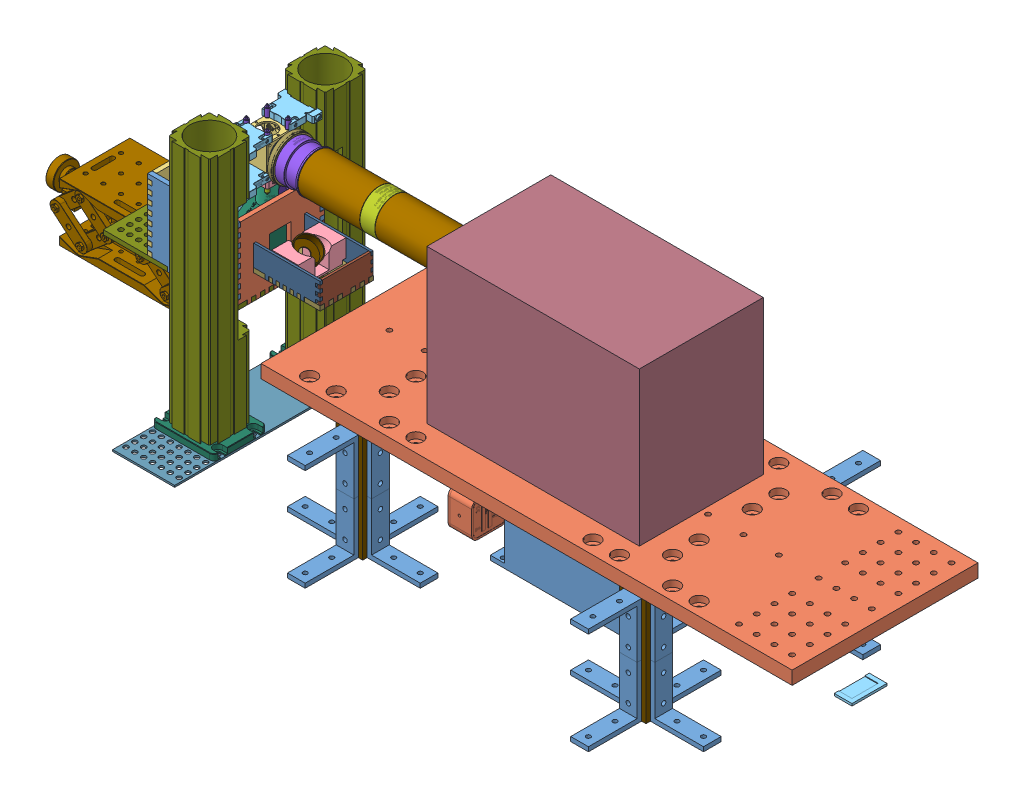
SolidWorks assembly Assembly4, configuration Default. Lengths in mm.
Overall size (1118.21 392.76 419.1).
142 component instances, 57 part files, 22 mates.
Components (placement in the parent):
- Laser Sub-Assembly-1: Laser Sub-Assembly [Default] at (5.2061 -104.2543 0) x (0 0 -1) z (1 0 0) size (111.76 88.9 267.97)
  - Laser-1: Laser [Default] at (0 -56.1594 0) x (0 0 1) z (-1 0 0) size (267.97 88.9 88.9)
  - SH05-Solidworks-1: SH05-Solidworks [Default] at (-45.783 38.7485 -122.8155) x (0 1 0) z (0 0 -1) size (57.1 81.96 34.87)
- Objective Sub-Assembly-1: Objective Sub-Assembly [Default] at (-505.0208 -286.1894 -114.3818) x (0 0 1) z (0 -1 0) size (106.71 57.63 128.02)
  - CM1-DCH-Solidworks-1: CM1-DCH-Solidworks [Web Assembly] at (114.3818 -34.6924 -438.5894) x (0 -1 0) z (0 0 1) size (38.1 45.72 38.1)
  - CP16-Solidworks-1: CP16-Solidworks [Default] at (116.5677 -16.5858 -398.1348) x (0 -1 0) z (0 0 1) size (41.22 40.64 8.89)
  - RCA2-Solidworks-1: RCA2-Solidworks [Default] at (123.339 -21.2203 -499.1988) x (0 -1 0) z (0 0 1) size (56.73 41.06 8.89)
  - RCA2-Solidworks-2: RCA2-Solidworks [Default] at (105.4247 -48.1644 -499.1988) x (0 1 0) z (0 0 1) size (56.73 41.06 8.89)
  - N40X-NIR-Solidworks-1: N40X-NIR-Solidworks [Default] at (114.3819 -34.6923 -375.0894) x (0 0 1) z (0.875921 0.482454 0) size (61.98 27.94 27.94)
  - RCA2-Solidworks-3: RCA2-Solidworks [Default] at (105.4247 -48.1644 -452.2088) x (0 1 0) z (0 0 1) size (56.73 41.06 8.89)
  - RCA2-Solidworks-4: RCA2-Solidworks [Default] at (123.339 -21.2203 -452.2088) x (0 -1 0) z (0 0 1) size (56.73 41.06 8.89)
  - ER1-Solidworks-1: ER1-Solidworks [Default] at (100.293 -20.9473 -404.3535) x (-0.183947 -0.982936 0) z (0.982936 -0.183947 0) size (5.99 30.48 5.99)
  - ER1-Solidworks-2: ER1-Solidworks [Default] at (130.5299 -50.7349 -404.3535) x (0.020475 -0.99979 0) z (0.99979 0.020475 0) size (5.99 30.48 5.99)
  - ER1-Solidworks-3: ER1-Solidworks [Default] at (100.0093 -51.1105 -404.3535) x (-0.386185 -0.922421 0) z (0.922421 -0.386185 0) size (5.99 30.48 5.99)
  - ER1-Solidworks-4: ER1-Solidworks [Default] at (129.6817 -21.2139 -404.3535) x (-0.579753 -0.814792 0) z (0.814792 -0.579753 0) size (5.99 30.48 5.99)
  - ER05-Solidworks-1: ER05-Solidworks [Default] at (129.9725 -48.2584 -461.5035) x (0.933397 0.358845 0) z (-0.358845 0.933397 0) size (5.99 17.78 5.99)
  - ER05-Solidworks-2: ER05-Solidworks [Default] at (97.9162 -50.199 -461.5035) x (-0.886919 0.461926 0) z (-0.461926 -0.886919 0) size (5.99 17.78 5.99)
  - ER05-Solidworks-3: ER05-Solidworks [Default] at (128.9134 -21.1707 -461.5035) x (-0.900043 -0.4358 0) z (0.4358 -0.900043 0) size (5.99 17.78 5.99)
  - ER05-Solidworks-4: ER05-Solidworks [Default] at (100.2773 -18.4261 -461.5035) x (0.989892 0.141823 0) z (-0.141823 0.989892 0) size (5.99 17.78 5.99)
- Tank Sub-Assembly-1: Tank Sub-Assembly [Default] at (-515.08 -14.5449 0) size (1033.25 293.3 151.27)
  - L490-Solidworks-1: L490-Solidworks [Default] at (-92.5657 -96.571 -35.1381) size (245.75 83.31 101.6)
  - Opticell-1: Opticell [Default] at (103.5741 151.5809 50.8) x (0 0 1) z (0.978619 -0.205679 0) size (76.36 12.75 129.72) (hidden)
  - Water Bath Sub-Assembly-1: Water Bath Sub-Assembly [Default] at origin size (285.88 143.69 129.57)
    - WB_0p125_SideLength-1: WB_0p125_SideLength [Default] at (107.95 57.023 -37.973) x (1 0 0) z (0 -1 0) size (101.6 3.17 36.83)
    - WB_0p125_SideLength-2: WB_0p125_SideLength [Default] at (107.95 57.023 35.052) x (1 0 0) z (0 -1 0) size (101.6 3.17 36.83)
    - WB_0p250_SideEnd-1: WB_0p250_SideEnd [Default] at (158.75 57.023 0.127) x (0 0 1) z (0 -1 0) size (76.2 3.17 36.83)
    - WB_0p250_SideBottom-1: WB_0p250_SideBottom [Default] at (108.077 35.433 0.127) size (101.6 6.35 76.2)
    - 500kHz-1: 500kHz [Default] at (-30.4673 57.15 0) x (1 0 0) z (0 -0.163379 0.986563) size (70.95 43.18 43.18)
    - 670kHz-1: 670kHz [Default] at (31.8426 57.15 0) x (0 -0.699517 -0.714616) z (1 0 0) size (68.07 68.07 113.8)
    - 300kHz-1: 300kHz [Default] at (-50.3061 44.1633 -1.0985) x (0 0 1) z (-1 0 0) size (91.44 91.44 114.81) (hidden)
    - HP Tx-1: HP Tx [Default] at (30.4173 57.15 0) x (0 -0.269446 0.963016) z (0 0.963016 0.269446) size (83.8 58.17 83.8)
    - WB_0p250_MainBottom-1: WB_0p250_MainBottom [Default] at origin size (190.5 6.35 127)
    - Cartrige-1: Cartrige [Default] at (82.8671 42.7355 -0.127) x (0 0 1) z (-1 0 0) size (50.29 3.17 25.4) (hidden)
    - Holder_500kHz-1: Holder_500kHz [Default] at (55.3093 57.15 0) x (0 0.524683 0.851298) z (0 -0.851298 0.524683) size (48.26 12.7 110.91)
    - PetriDish-1: PetriDish [Default] at (97.5883 57.023 -0.508) x (-0.361353 0.253022 -0.897443) z (0.735142 -0.514752 -0.441131) size (35.56 11.05 35.56)
    - WB_0p250_MainWall-1: WB_0p250_MainWall [Default] at (0 53.975 63.5) x (-1 0 0) z (0 -1 0) size (127 6.35 107.95)
    - WB_0p250_MainWall-2: WB_0p250_MainWall [Default] at (0 53.975 -57.15) x (-1 0 0) z (0 -1 0) size (127 6.35 107.95)
    - WB_0p250_MainLengthOverhangHoleV3-1: WB_0p250_MainLengthOverhangHoleV3 [Default] at (57.15 53.975 0) x (0 0 -1) z (0 -1 0) size (127 6.35 107.95)
    - WB_0p250_MainLengthOverhangV3-1: WB_0p250_MainLengthOverhangV3 [Default] at (-63.5 53.975 0) x (0 0 -1) z (0 -1 0) size (127 6.35 107.95)
    - CartridgeHolder_V5-1: CartridgeHolder_V5 [Default] at (100.9425 57.023 -0.1905) x (0 0 -1) z (1 0 0) size (69.22 30.48 22.23) (hidden)
    - PetriHolderV3-1: PetriHolderV3 [Default] at (97.5883 57.023 -0.508) x (0 0 -1) z (1 0 0) size (68.58 30.48 38.1)
  - CartrigeHolder-1: CartrigeHolder [Default] at (47.2922 57.163 6.223) x (0 0 -1) z (1 0 0) size (82.55 22.23 25.4) (hidden)
  - PetriDish-1: PetriDish [Default] at (36.8111 56.7801 50.8) x (0 0 1) z (-0.866025 0.5 0) size (35.56 11.05 35.56) (hidden)
  - Cartrige-1: Cartrige [Default] at (820.7316 -148.0288 -62.6211) x (0 0 1) z (-1 0 0) size (50.29 3.17 25.4)
  - PetriHolder-1: PetriHolder [Default] at (79.8565 60.1253 -3.1464) x (0.866025 -0.5 0) z (0 0 1) size (38.1 29.14 68.58) (hidden)
  - PetriDish-2: PetriDish [Default] at (79.8565 60.1253 -3.1464) x (0.85505 -0.493663 0.158703) z (-0.137441 0.079352 0.987326) size (35.56 11.05 35.56) (hidden)
- Camera Sub-Assembly-1: Camera Sub-Assembly [Default] at (-451.2785 152.4 0) x (0 0 1) z (-1 0 0) size (71.93 71.93 298.88)
  - SM2NFM2-Solidworks-1: SM2NFM2-Solidworks [Default] at (0 0 -285.6832) x (0 1 0) z (-1 0 0) size (63.5 16.37 63.5)
  - TTL200-S8-Solidworks-1: TTL200-S8-Solidworks [Default] at (0 0 -152.5317) size (55.88 55.88 28)
  - SM2V15-Solidworks-1: SM2V15-Solidworks [Default] at (18.0496 -29.8565 -288.422) x (0 0 -1) z (0.951776 0.306793 0) size (51.56 57.15 57.15)
  - SM2M35-Solidworks-1: SM2M35-Solidworks [Default] at (-10.7846 9.351 -219.5042) x (0.99081 -0.135264 0) z (0 0 1) size (55.88 55.88 88.9)
  - SM2M35-Solidworks-2: SM2M35-Solidworks [Default] at (-11.8362 7.9783 -108.9542) x (0.999895 -0.014459 0) z (0 0 1) size (55.88 55.88 88.9)
  - SM2V15-Solidworks-2: SM2V15-Solidworks [Default] at (-9.1968 -33.7176 -16.6413) x (0 0 1) z (-0.999373 0.035397 0) size (51.56 57.15 57.15)
  - SM1T2-Solidworks-1: SM1T2-Solidworks [Default] at (0 0 1.778) x (0.997143 -0.075539 0) z (0 0 1) size (31.75 31.75 12.7)
  - SM2A6-Solidworks-2: SM2A6-Solidworks [Default] at (0 0 -9.144) size (51.69 51.69 5.08)
  - SM2D25D-Solidworks-1: SM2D25D-Solidworks [Default] at (-6.3593 1.1475 -12.9462) x (-1 0 0) z (0 0 -1) size (60.96 60.96 12.32)
- hpvx2-1: hpvx2 [Default] at origin size (311.15 228.6 177.8)
- Small Condenser Adjustable Sub-Assembly-1: Small Condenser Adjustable Sub-Assembly [Default] at (-505.8885 -28.0543 -20.3199) x (0 -1 0) z (0 0 -1) size (218.8 286.9 106.71) (hidden)
  - LB1437-Solidworks-1: LB1437-Solidworks [Default] at (76.2 -223.413 -20.3199) x (0.879994 0 -0.474985) z (0 -1 0) size (25.4 25.4 3.05)
  - LB1761-Solidworks-1: LB1761-Solidworks [Default] at (76.2 -78.613 -20.3199) x (0.962182 0 -0.272406) z (0 -1 0) size (25.4 25.4 8.98)
  - SM1L40-Solidworks-1: SM1L40-Solidworks [Default] at (78.3398 -122.5422 -22.1696) x (-0.992854 0 -0.119336) z (0 1 0) size (30.48 30.48 105.41)
  - CSA1003-Solidworks-1: CSA1003-Solidworks [Default] at (47.6181 -122.449 -34.035) x (0 -1 0) z (0 0 1) size (71.12 13.97 71.12)
  - LCP02-Solidworks-1: LCP02-Solidworks [Default] at (20.32 -35.5599 -20.32) x (0 0 -1) z (1 0 0) size (70.75 70.61 12.7)
  - ER1-Solidworks-1: ER1-Solidworks [Default] at (36.8841 -51.9737 -4.6825) x (0 -0.925141 -0.379624) z (0 -0.379624 0.925141) size (5.99 30.48 5.99)
  - ER1-Solidworks-3: ER1-Solidworks [Default] at (36.8841 -50.6608 -33.7724) x (0 -0.769482 0.638668) z (0 0.638668 0.769482) size (5.99 30.48 5.99)
  - ER1-Solidworks-4: ER1-Solidworks [Default] at (41.8559 -21.5595 -36.5057) x (0 -0.998351 -0.057413) z (0 0.057413 -0.998351) size (5.99 30.48 5.99)
  - CPB1-Solidworks-2: CPB1-Solidworks [Default] at (105.41 -256.9972 27.3051) x (0 0 1) z (0 -1 0) size (95.25 10.79 15.24)
  - CP08-Solidworks-2: CP08-Solidworks [Default] at (76.2 -263.9822 -20.3199) x (0 0 -1) z (0 1 0) size (41.5 40.64 8.89)
  - SM1T2-Solidworks-1: SM1T2-Solidworks [Default] at (76.2 -248.6152 -20.3199) x (0.998592 0 -0.053039) z (0 1 0) size (31.75 31.75 12.7)
  - SM1L25-Solidworks-1: SM1L25-Solidworks [Default] at (139.9124 -186.275 -15.6668) x (0 -1 0) z (-0.806632 0 -0.591053) size (67.31 30.48 30.48)
  - CPB1-Solidworks-3: CPB1-Solidworks [Default] at (105.41 -62.23 27.3051) x (0 0 1) z (0 -1 0) size (95.25 10.79 15.24)
  - CP08-Solidworks-3: CP08-Solidworks [Default] at (76.2 -69.215 -20.3199) x (0 0 -1) z (0 1 0) size (41.5 40.64 8.89)
  - KCB1-Solidworks-2: KCB1-Solidworks [Default] at (100.33 -11.43 3.8101) x (-1 0 0) z (0 -1 0) size (51.13 48.26 51.1)
  - ER1-Solidworks-6: ER1-Solidworks [Default] at (36.8841 -20.7263 -3.7781) x (0 -0.795862 0.605478) z (0 0.605478 0.795862) size (5.99 30.48 5.99)
  - RCA2-Solidworks-1: RCA2-Solidworks [Default] at (68.2294 -49.0321 -29.2771) x (0 1 0) z (-1 0 0) size (56.73 41.06 8.89)
  - RCA2-Solidworks-2: RCA2-Solidworks [Default] at (68.2294 -22.0879 -11.3628) x (0 -1 0) z (-1 0 0) size (56.73 41.06 8.89)
  - TR075-Solidworks-1: TR075-Solidworks [Default] at (105.41 -263.9822 17.7801) x (0 0 -1) z (0 -1 0) size (12.67 19.05 12.87)
  - TR075-Solidworks-2: TR075-Solidworks [Default] at (143.51 -263.9822 17.7801) x (0 0 1) z (0 -1 0) size (12.67 19.05 12.87)
  - PH1.5-Solidworks-1: PH1.5-Solidworks [Default] at (136.906 -263.9822 17.7801) x (0 0 1) z (0 -1 0) size (25 38.71 35.41)
  - ER05-Solidworks-1: ER05-Solidworks [Default] at (92.6015 -68.5259 -5.9839) x (0.310188 0 -0.950675) z (0.950675 0 0.310188) size (5.99 17.78 5.99)
  - ER05-Solidworks-2: ER05-Solidworks [Default] at (59.8613 -68.5259 -4.5371) x (-0.22668 0 0.973969) z (-0.973969 0 -0.22668) size (5.99 17.78 5.99)
  - ER05-Solidworks-3: ER05-Solidworks [Default] at (92.2659 -68.5259 -34.1935) size (5.99 17.78 5.99)
  - ER05-Solidworks-4: ER05-Solidworks [Default] at (59.7556 -68.5259 -34.7555) x (-0.375833 0 0.926687) z (-0.926687 0 -0.375833) size (5.99 17.78 5.99)
  - SM1D12D-Solidworks-1: SM1D12D-Solidworks [Default] at (81.3975 -244.783 -22.8892) x (0.973299 0 -0.22954) z (0 1 0) size (35.81 35.81 11.94)
  - SM1D12D-Solidworks-2: SM1D12D-Solidworks [Default] at (70.9424 -73.1298 -22.7639) x (-0.788375 0 -0.615195) z (0 1 0) size (35.81 35.81 11.94)
  - ER1-Solidworks-9: ER1-Solidworks [Default] at (15.1859 -4.2179 -49.5429) x (0 0.95877 -0.284182) z (0 0.284182 0.95877) size (5.99 30.48 5.99)
  - ER1-Solidworks-10: ER1-Solidworks [Default] at (15.1859 -64.6339 -49.076) x (0 0.993069 0.117534) z (0 -0.117534 0.993069) size (5.99 30.48 5.99)
  - ER1-Solidworks-11: ER1-Solidworks [Default] at (15.1859 -4.6008 10.8986) x (0 0.995869 0.090807) z (0 -0.090807 0.995869) size (5.99 30.48 5.99)
  - ER1-Solidworks-12: ER1-Solidworks [Default] at (15.1859 -64.2349 10.4858) x (0 0.96466 -0.263499) z (0 0.263499 0.96466) size (5.99 30.48 5.99)
  - BeckmanCondenser-1: BeckmanCondenser [Default] at (7.0104 -35.56 -20.3199) x (0 -1 0) z (0 0 -1) size (71.12 69.85 91.44)
- Table SubAssembly-1: Table SubAssembly [Default] at (-507.922 -162.9537 0.0025) x (0 0 -1) z (1 0 0) size (355.6 366.78 89.6)
  - Table-1: Table [Default] at origin size (355.6 2.54 88.9)
  - XT66P1-Solidworks-1: XT66P1-Solidworks [Default] at (-83.0224 2.286 37.592) x (-1 0 0) z (0 0 -1) size (76.2 8.89 89.28)
  - XT66P1-Solidworks-2: XT66P1-Solidworks [Default] at (83.0224 2.286 37.592) size (76.2 8.89 89.28)
  - KCB1-Solidworks-1: KCB1-Solidworks [Default] at (-24.13 99.7796 13.4747) x (0.000001 0 1) z (0 1 0) size (51.13 48.26 51.1) (hidden)
  - RCA1-Solidworks-1: RCA1-Solidworks [Default] at (-24.2926 205.6203 66.0649) x (0 0 -1) z (0 -1 0) size (56.5 73.55 8.89) (hidden)
  - RCA1-Solidworks-2: RCA1-Solidworks [Default] at (24.2926 108.2389 66.0649) x (0 0 -1) z (0 1 0) size (56.5 73.55 8.89) (hidden)
  - XT66-500-modified-1: XT66-500-modified [Default] at (-83.0224 511.176 37.592) x (0 0 -1) z (0 -1 0) size (66.02 67.06 355.6)
  - XT66-500-modified-2: XT66-500-modified [Default] at (83.0224 511.176 37.592) x (0 0 1) z (0 -1 0) size (66.02 67.06 355.6)
- TR1-Solidworks-1: TR1-Solidworks [Default] at (-241.9063 -160.4137 -38.1) size (12.67 29.6 12.87)
- Full Assembly Total Support-1: Full Assembly Total Support [Default] at (193.3222 -162.9537 -53.958) size (762 171.45 419.1)
  - Post SubAssembly-1: Post SubAssembly [Default] at (-412.4306 0 168.258) size (190.5 152.4 190.5)
    - Post-1: Post [Default] at origin size (38.1 152.4 38.1)
    - Hinge-1: Hinge [Default] at (-25.4 6.35 0) x (0 0 -1) z (0 -1 0) size (25.4 76.2 76.2)
    - Hinge-2: Hinge [Default] at (0 6.35 25.4) x (-1 0 0) z (0 -1 0) size (25.4 76.2 76.2)
    - Hinge-3: Hinge [Default] at (25.4 6.35 0) x (0 0 1) z (0 -1 0) size (25.4 76.2 76.2)
    - Hinge-4: Hinge [Default] at (0 6.35 -25.4) x (1 0 0) z (0 -1 0) size (25.4 76.2 76.2)
    - Hinge-5: Hinge [Default] at (25.4 146.05 0) x (0 0 1) z (-1 0 0) size (25.4 76.2 76.2)
    - Hinge-7: Hinge [Default] at (-25.4 146.05 0) x (0 0 -1) z (1 0 0) size (25.4 76.2 76.2)
    - Hinge-8: Hinge [Default] at (0 146.05 25.4) x (-1 0 0) z (0 0 -1) size (25.4 76.2 76.2)
    - Hinge-9: Hinge [Default] at (0 146.05 -25.4) size (25.4 76.2 76.2)
  - Post SubAssembly-2: Post SubAssembly [Default] at (-412.4306 0 -60.342) size (190.5 152.4 190.5)
    - Post-1: Post [Default] at origin size (38.1 152.4 38.1)
    - Hinge-1: Hinge [Default] at (-25.4 6.35 0) x (0 0 -1) z (0 -1 0) size (25.4 76.2 76.2)
    - Hinge-2: Hinge [Default] at (0 6.35 25.4) x (-1 0 0) z (0 -1 0) size (25.4 76.2 76.2)
    - Hinge-3: Hinge [Default] at (25.4 6.35 0) x (0 0 1) z (0 -1 0) size (25.4 76.2 76.2)
    - Hinge-4: Hinge [Default] at (0 6.35 -25.4) x (1 0 0) z (0 -1 0) size (25.4 76.2 76.2)
    - Hinge-5: Hinge [Default] at (25.4 146.05 0) x (0 0 1) z (-1 0 0) size (25.4 76.2 76.2)
    - Hinge-7: Hinge [Default] at (-25.4 146.05 0) x (0 0 -1) z (1 0 0) size (25.4 76.2 76.2)
    - Hinge-8: Hinge [Default] at (0 146.05 25.4) x (-1 0 0) z (0 0 -1) size (25.4 76.2 76.2)
    - Hinge-9: Hinge [Default] at (0 146.05 -25.4) size (25.4 76.2 76.2)
  - Post SubAssembly-3: Post SubAssembly [Default] at (-6.0306 0 168.258) size (190.5 152.4 190.5)
    - Post-1: Post [Default] at origin size (38.1 152.4 38.1)
    - Hinge-1: Hinge [Default] at (-25.4 6.35 0) x (0 0 -1) z (0 -1 0) size (25.4 76.2 76.2)
    - Hinge-2: Hinge [Default] at (0 6.35 25.4) x (-1 0 0) z (0 -1 0) size (25.4 76.2 76.2)
    - Hinge-3: Hinge [Default] at (25.4 6.35 0) x (0 0 1) z (0 -1 0) size (25.4 76.2 76.2)
    - Hinge-4: Hinge [Default] at (0 6.35 -25.4) x (1 0 0) z (0 -1 0) size (25.4 76.2 76.2)
    - Hinge-5: Hinge [Default] at (25.4 146.05 0) x (0 0 1) z (-1 0 0) size (25.4 76.2 76.2)
    - Hinge-7: Hinge [Default] at (-25.4 146.05 0) x (0 0 -1) z (1 0 0) size (25.4 76.2 76.2)
    - Hinge-8: Hinge [Default] at (0 146.05 25.4) x (-1 0 0) z (0 0 -1) size (25.4 76.2 76.2)
    - Hinge-9: Hinge [Default] at (0 146.05 -25.4) size (25.4 76.2 76.2)
  - Post SubAssembly-4: Post SubAssembly [Default] at (-6.0306 0 -60.342) size (190.5 152.4 190.5)
    - Post-1: Post [Default] at origin size (38.1 152.4 38.1)
    - Hinge-1: Hinge [Default] at (-25.4 6.35 0) x (0 0 -1) z (0 -1 0) size (25.4 76.2 76.2)
    - Hinge-2: Hinge [Default] at (0 6.35 25.4) x (-1 0 0) z (0 -1 0) size (25.4 76.2 76.2)
    - Hinge-3: Hinge [Default] at (25.4 6.35 0) x (0 0 1) z (0 -1 0) size (25.4 76.2 76.2)
    - Hinge-4: Hinge [Default] at (0 6.35 -25.4) x (1 0 0) z (0 -1 0) size (25.4 76.2 76.2)
    - Hinge-5: Hinge [Default] at (25.4 146.05 0) x (0 0 1) z (-1 0 0) size (25.4 76.2 76.2)
    - Hinge-7: Hinge [Default] at (-25.4 146.05 0) x (0 0 -1) z (1 0 0) size (25.4 76.2 76.2)
    - Hinge-8: Hinge [Default] at (0 146.05 25.4) x (-1 0 0) z (0 0 -1) size (25.4 76.2 76.2)
    - Hinge-9: Hinge [Default] at (0 146.05 -25.4) size (25.4 76.2 76.2)
  - Camera Shelf Full Support v2-1: Camera Shelf Full Support v2 [Default] at (-158.3164 152.4 53.958) size (762 19.05 266.7)
Mates (geometry in assembly coordinates):
- Concentric5: concentric anti-aligned: cylinder of Camera Sub-Assembly-1/SM2M35-Solidworks-1 through (-240.9318 152.4 0) axis (-1 0 0) radius 27.94; cylinder of hpvx2-1 through (-152.4 152.4 0) axis (1 0 0) radius 29.1375
- Coincident10: coincident anti-aligned: plane of Camera Sub-Assembly-1/SM2NFM2-Solidworks-1 through (-158.75 152.4713 0.0001) normal (1 0 0); plane of hpvx2-1 through (-158.75 152.4 0) normal (-1 0 0)
- Coincident13: coordinate: point of hpvx2-1; point of assembly
- Concentric9: concentric anti-aligned: circle of Small Condenser Adjustable Sub-Assembly-1/CPB1-Solidworks-2; circle of TR1-Solidworks-1
- Parallel16: parallel aligned: plane of Laser Sub-Assembly-1/Laser-1 through (5.2061 -71.5137 0) normal (0 1 0); plane of hpvx2-1 through (0 228.6 0) normal (0 1 0)
- Parallel17: parallel aligned: plane of Laser Sub-Assembly-1/Laser-1 through (5.2061 -71.5137 0) normal (0 1 0); plane of Tank Sub-Assembly-1/L490-Solidworks-1 through (-565.88 -14.5449 25.4) normal (0 1 0)
- Coincident44: coincident aligned: plane of Camera Sub-Assembly-1 through (-451.2785 152.4 0) normal (0 0 1); plane of assembly through (0 0 0) normal (0 0 1)
- Concentric11: concentric anti-aligned: circle of Objective Sub-Assembly-1/CM1-DCH-Solidworks-1; cylinder of Camera Sub-Assembly-1/SM2M35-Solidworks-2 through (-351.4818 152.4 0) axis (-1 0 0) radius 27.94
- Concentric12: concentric aligned: circle of Objective Sub-Assembly-1/CM1-DCH-Solidworks-1; circle of Small Condenser Adjustable Sub-Assembly-1/CSA1003-Solidworks-1
- Parallel18: parallel anti-aligned: plane of hpvx2-1 through (-152.4 228.6 88.9) normal (0 0 1); plane of Small Condenser Adjustable Sub-Assembly-1/CSA1003-Solidworks-1 through (-505.8885 -28.0543 -35.56) normal (0 0 -1)
- Coincident50: coincident anti-aligned: plane of Objective Sub-Assembly-1/CM1-DCH-Solidworks-1 through (-451.2785 133.35 19.05) normal (1 0 0); plane of Camera Sub-Assembly-1/SM1T2-Solidworks-1 through (-451.2785 151.3738 13.5456) normal (-1 0 0)
- Coincident54: coincident aligned: plane of hpvx2-1 through (0 0 0) normal (0 0 1); plane of Full Assembly Total Support-1/Camera Shelf Full Support v2-1 through (35.0058 -10.5537 0) normal (0 0 1)
- Concentric13: concentric anti-aligned: cylinder of Laser Sub-Assembly-1/Laser-1 through (5.2061 -104.2543 0) axis (1 0 0) radius 15.24; cylinder of Small Condenser Adjustable Sub-Assembly-1/SM1L40-Solidworks-1 through (-433.6255 -104.2543 0) axis (-1 0 0) radius 15.24
- Coincident57: coincident anti-aligned: plane of Table SubAssembly-1/Table-1 through (-507.922 -160.4137 0.0025) normal (0 1 0); plane of TR1-Solidworks-1 through (-236.077 -160.4137 -38.1) normal (0 -1 0)
- Coincident59: coincident aligned: plane of Table SubAssembly-1/Table-1 through (-507.922 -162.9537 0.0025) normal (0 -1 0); plane of Full Assembly Total Support-1/Post SubAssembly-1/Hinge-2 through (-231.8084 -162.9537 209.55) normal (0 -1 0)
- Coincident67: coincident anti-aligned: plane of Objective Sub-Assembly-1/RCA2-Solidworks-2 through (-485.174 171.45 -50) normal (0 0 -1); plane of ? through (-490.3452 348.2213 -50) normal (0 0 1)
- Coincident68: coincident anti-aligned: plane of Objective Sub-Assembly-1/RCA2-Solidworks-2 through (-488.0055 171.45 -53.3557) normal (0.707107 0 0.707107); plane of ? through (-490.3452 348.2213 -51.016) normal (-0.707107 0 -0.707107)
- Coincident70: coincident anti-aligned: plane of Laser Sub-Assembly-1/Laser-1 through (5.2061 -160.4137 0) normal (0 -1 0); plane of Table SubAssembly-1/Table-1 through (-507.922 -160.4137 0.0025) normal (0 1 0)
- Distance3: distance = 30.6197 mm anti-aligned: plane of Small Condenser Adjustable Sub-Assembly-1/BeckmanCondenser-1 through (-470.3285 34.7853 0) normal (0 1 0); plane of Objective Sub-Assembly-1/N40X-NIR-Solidworks-1 through (-506.3907 65.405 -19.8629) normal (0 -1 0)
- Distance4: distance = 127 mm anti-aligned: plane of Tank Sub-Assembly-1/L490-Solidworks-1 through (-630.3627 -87.5132 25.4) normal (1 0 0); plane of ? through (-503.3627 348.2213 -103.0225) normal (-1 0 0)
- Coincident71: coincident: plane of Tank Sub-Assembly-1/Water Bath Sub-Assembly-1 through (-493.2027 8.4597 0) normal (0 0 -1); plane of assembly through (0 0 0) normal (0 0 1)
- Coincident72: coincident aligned: plane of Tank Sub-Assembly-1/Water Bath Sub-Assembly-1/WB_0p250_MainBottom-1 through (-515.08 -14.5449 0) normal (0 0 1); plane of assembly through (0 0 0) normal (0 0 1)
